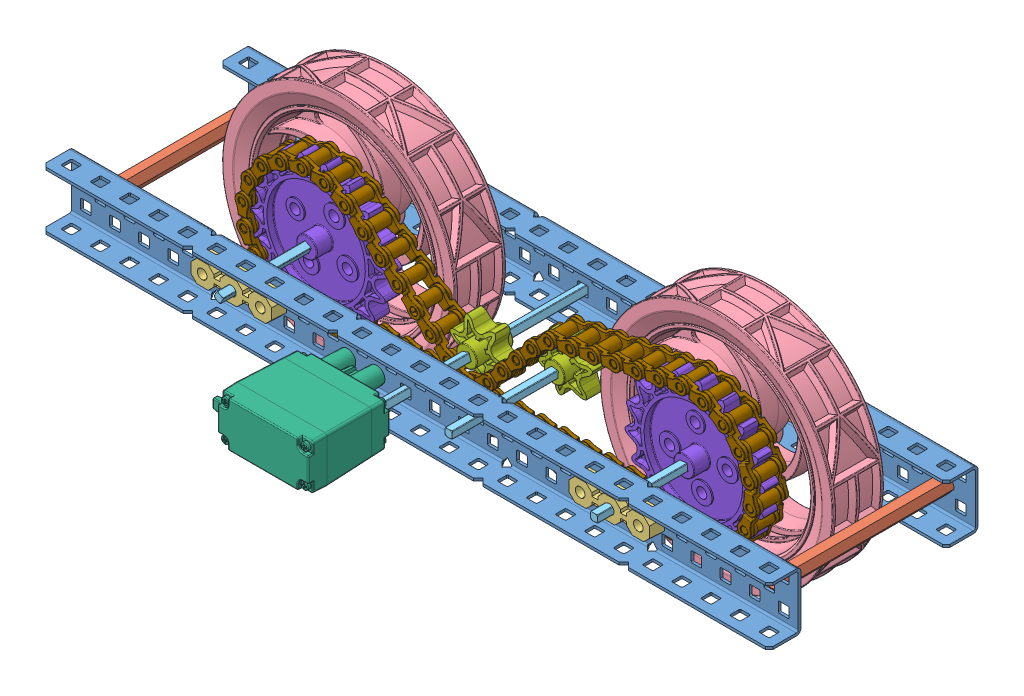
SolidWorks assembly Chassis-NoMates, configuration Default. Lengths in mm.
Overall size (317.5 140.41 141.11).
74 component instances, 9 part files, 0 mates.
Components (placement in the parent):
- BaseUC-4: BaseUC [Default] at (-291.0348 15.6006 0) x (1 0 0) z (0 1 0) size (317.5 13.87 25.4)
- BEAM-3000-7: BEAM-3000 [Default] at (-304.8 12.7 -39.2684) x (1 0 0) z (0 -1 0) size (7.34 77.08 7.34)
- BEAM-3000-8: BEAM-3000 [Default] at (-12.7 12.7 -39.2684) x (-0.63784 -0.770169 0) z (-0.770169 0.63784 0) size (7.34 77.08 7.34)
- BaseUC-7: BaseUC [Default] at (-291.0348 15.6006 -77.3684) x (1 0 0) z (0 1 0) size (317.5 13.87 25.4)
- BEARING-FLAT-5: BEARING-FLAT [Default] at (-49.784 25.4 88.9762) x (0 0 -1) z (0 1 0) size (7.04 35.56 10.16)
- BEARING-FLAT-6: BEARING-FLAT [Default] at (-214.884 25.4 88.9762) x (0 0 -1) z (0 1 0) size (7.04 35.56 10.16)
- BEARING-FLAT-7: BEARING-FLAT [Default] at (-49.784 25.4 11.6078) x (0 0 -1) z (0 1 0) size (7.04 35.56 10.16)
- BEARING-FLAT-8: BEARING-FLAT [Default] at (-214.884 25.4 11.6078) x (0 0 -1) z (0 1 0) size (7.04 35.56 10.16)
- VEX-MEDIUM-WHEEL-3: VEX-MEDIUM-WHEEL [Default] at (-37.1315 -9.2154 -55.044) x (0.998133 0.061083 0) z (0 0 1) size (132.42 132.57 22.31)
- VEX-MEDIUM-WHEEL-4: VEX-MEDIUM-WHEEL [Default] at (-202.5787 -9.8231 -55.044) x (0.998965 0.045481 0) z (0 0 1) size (132.42 132.57 22.31)
- SHAFT-4000-1: SHAFT-4000 [Default] at (-241.3972 12.7906 -38.9947) x (0.456181 0.889887 0) z (0 0 1) size (4.18 4.18 101.81)
- SHAFT-4000-2: SHAFT-4000 [Default] at (-76.5518 12.5236 -38.1812) x (-0.999953 -0.009699 0) z (0 0 1) size (4.18 4.18 101.81)
- SHAFT-4000-3: SHAFT-4000 [Default] at (-132.8293 19.7739 -30.9) size (4.18 4.18 101.81)
- SHAFT-4000-4: SHAFT-4000 [Default] at (-171.4187 6.3323 -30.9) x (-0.963526 -0.267616 0) z (0 0 1) size (4.18 4.18 101.81)
- VEX-2WIRE-MOTOR-1: VEX-2WIRE-MOTOR [Default] at (-182.5798 6.35 43.2) size (46.4 20 51.81)
- sprocket-hs-06-tooth-1: sprocket-hs-06-tooth [Default] at (-171.4187 6.3323 -34.515) x (0.920352 0.391092 0) z (0 0 1) size (21.52 24.74 15.88)
- sprocket-hs-18-tooth-1: sprocket-hs-18-tooth [Default] at (-241.3 12.7 -34.515) x (0.897713 -0.440581 0) z (0 0 1) size (60.62 61.51 15.88)
- sprocket-hs-18-tooth-2: sprocket-hs-18-tooth [Default] at (-76.2 12.7 -34.193) x (0.11417 -0.993461 0) z (0 0 1) size (60.62 61.51 15.88)
- sprocket-hs-06-tooth-2: sprocket-hs-06-tooth [Default] at (-132.8293 19.7739 -34.193) x (0.976296 -0.21644 0) z (0 0 1) size (21.52 24.74 15.88)
- chain-hs-link-1: chain-hs-link [Default] at (-202.2568 17.8785 -29.705) x (0.779269 -0.62669 0) z (0.62669 0.779269 0) size (15.79 14.22 6)
- chain-hs-link-3: chain-hs-link [Default] at (-209.8931 24.0197 -29.705) x (0.779269 -0.62669 0) z (0.62669 0.779269 0) size (15.79 14.22 6)
- chain-hs-link-4: chain-hs-link [Default] at (-217.5294 30.1608 -29.705) x (0.779269 -0.62669 0) z (0.62669 0.779269 0) size (15.79 14.22 6)
- chain-hs-link-5: chain-hs-link [Default] at (-225.2134 36.2422 -29.705) x (0.784132 -0.620594 0) z (0.620594 0.784132 0) size (15.79 14.22 6)
- chain-hs-link-6: chain-hs-link [Default] at (-234.1156 40.3382 -29.705) x (0.908451 -0.417991 0) z (0.417991 0.908451 0) size (15.79 14.22 6)
- chain-hs-link-7: chain-hs-link [Default] at (-243.879 41.1761 -29.705) x (0.996338 -0.0855 0) z (0.0855 0.996338 0) size (15.79 14.22 6)
- chain-hs-link-8: chain-hs-link [Default] at (-253.3489 38.6566 -29.705) x (0.966384 0.257104 0) z (-0.257104 0.966384 0) size (15.79 14.22 6)
- chain-hs-link-9: chain-hs-link [Default] at (-261.4052 33.0779 -29.705) x (0.822131 0.569299 0) z (-0.569299 0.822131 0) size (15.79 14.22 6)
- chain-hs-link-10: chain-hs-link [Default] at (-267.0951 25.0997 -29.705) x (0.58064 0.81416 0) z (-0.81416 0.58064 0) size (15.79 14.22 6)
- chain-hs-link-11: chain-hs-link [Default] at (-269.7456 15.6656 -29.705) x (0.270475 0.962727 0) z (-0.962727 0.270475 0) size (15.79 14.22 6)
- chain-hs-link-12: chain-hs-link [Default] at (-269.0432 5.8915 -29.705) x (-0.071681 0.997428 0) z (-0.997428 -0.071681 0) size (15.79 14.22 6)
- chain-hs-link-13: chain-hs-link [Default] at (-265.0709 -3.0666 -29.705) x (-0.405359 0.914158 0) z (-0.914158 -0.405359 0) size (15.79 14.22 6)
- chain-hs-link-14: chain-hs-link [Default] at (-258.2987 -10.1493 -29.705) x (-0.691093 0.722766 0) z (-0.722766 -0.691093 0) size (15.79 14.22 6)
- chain-hs-link-15: chain-hs-link [Default] at (-249.5274 -14.5187 -29.705) x (-0.895088 0.44589 0) z (-0.44589 -0.895088 0) size (15.79 14.22 6)
- chain-hs-link-16: chain-hs-link [Default] at (-239.8 -15.7032 -29.705) x (-0.992667 0.120879 0) z (-0.120879 -0.992667 0) size (15.79 14.22 6)
- chain-hs-link-17: chain-hs-link [Default] at (-230.0006 -15.7032 -29.705) x (-1 0 0) z (0 -1 0) size (15.79 14.22 6)
- chain-hs-link-18: chain-hs-link [Default] at (-220.2013 -15.7032 -29.705) x (-1 0 0) z (0 -1 0) size (15.79 14.22 6)
- chain-hs-link-19: chain-hs-link [Default] at (-210.402 -15.7032 -29.705) x (-1 0 0) z (0 -1 0) size (15.79 14.22 6)
- chain-hs-link-20: chain-hs-link [Default] at (-200.6027 -15.7032 -29.705) x (-1 0 0) z (0 -1 0) size (15.79 14.22 6)
- chain-hs-link-21: chain-hs-link [Default] at (-190.8033 -15.7032 -29.705) x (-1 0 0) z (0 -1 0) size (15.79 14.22 6)
- chain-hs-link-22: chain-hs-link [Default] at (-181.004 -15.7032 -29.705) x (-1 0 0) z (0 -1 0) size (15.79 14.22 6)
- chain-hs-link-23: chain-hs-link [Default] at (-171.2047 -15.7032 -29.705) x (-1 0 0) z (0 -1 0) size (15.79 14.22 6)
- chain-hs-link-24: chain-hs-link [Default] at (-161.4054 -15.7032 -29.705) x (-1 0 0) z (0 -1 0) size (15.79 14.22 6)
- chain-hs-link-25: chain-hs-link [Default] at (-151.6061 -15.7032 -29.705) x (-1 0 0) z (0 -1 0) size (15.79 14.22 6)
- chain-hs-link-26: chain-hs-link [Default] at (-141.8067 -15.7032 -29.705) x (-1 0 0) z (0 -1 0) size (15.79 14.22 6)
- chain-hs-link-27: chain-hs-link [Default] at (-132.0074 -15.7032 -29.705) x (-1 0 0) z (0 -1 0) size (15.79 14.22 6)
- chain-hs-link-28: chain-hs-link [Default] at (-122.2081 -15.7032 -29.705) x (-1 0 0) z (0 -1 0) size (15.79 14.22 6)
- chain-hs-link-29: chain-hs-link [Default] at (-112.4088 -15.7032 -29.705) x (-1 0 0) z (0 -1 0) size (15.79 14.22 6)
- chain-hs-link-30: chain-hs-link [Default] at (-102.6094 -15.7032 -29.705) x (-1 0 0) z (0 -1 0) size (15.79 14.22 6)
- chain-hs-link-31: chain-hs-link [Default] at (-92.8101 -15.7032 -29.705) x (-1 0 0) z (0 -1 0) size (15.79 14.22 6)
- chain-hs-link-32: chain-hs-link [Default] at (-83.0108 -15.7032 -29.705) x (-1 0 0) z (0 -1 0) size (15.79 14.22 6)
- chain-hs-link-33: chain-hs-link [Default] at (-73.2127 -15.5457 -29.705) x (-0.999871 -0.016075 0) z (0.016075 -0.999871 0) size (15.79 14.22 6)
- chain-hs-link-34: chain-hs-link [Default] at (-63.7916 -12.8494 -29.705) x (-0.961403 -0.275144 0) z (0.275144 -0.961403 0) size (15.79 14.22 6)
- chain-hs-link-35: chain-hs-link [Default] at (-55.8475 -7.1121 -29.705) x (-0.810681 -0.585488 0) z (0.585488 -0.810681 0) size (15.79 14.22 6)
- chain-hs-link-36: chain-hs-link [Default] at (-50.326 0.9836 -29.705) x (-0.563464 -0.826141 0) z (0.826141 -0.563464 0) size (15.79 14.22 6)
- chain-hs-link-37: chain-hs-link [Default] at (-47.8842 10.4738 -29.705) x (-0.249177 -0.968458 0) z (0.968458 -0.249177 0) size (15.79 14.22 6)
- chain-hs-link-38: chain-hs-link [Default] at (-48.8129 20.229 -29.705) x (0.09477 -0.995499 0) z (0.995499 0.09477 0) size (15.79 14.22 6)
- chain-hs-link-39: chain-hs-link [Default] at (-53.0014 29.0881 -29.705) x (0.427436 -0.904046 0) z (0.904046 0.427436 0) size (15.79 14.22 6)
- chain-hs-link-40: chain-hs-link [Default] at (-59.9513 35.9964 -29.705) x (0.709224 -0.704984 0) z (0.704984 0.709224 0) size (15.79 14.22 6)
- chain-hs-link-41: chain-hs-link [Default] at (-68.8353 40.1318 -29.705) x (0.906593 -0.422007 0) z (0.422007 0.906593 0) size (15.79 14.22 6)
- chain-hs-link-42: chain-hs-link [Default] at (-78.596 41.002 -29.705) x (0.99605 -0.088798 0) z (0.088798 0.99605 0) size (15.79 14.22 6)
- chain-hs-link-43: chain-hs-link [Default] at (-88.2359 39.2421 -29.705) x (0.983741 0.179593 0) z (-0.179593 0.983741 0) size (15.79 14.22 6)
- chain-hs-link-44: chain-hs-link [Default] at (-97.8402 37.2967 -29.705) x (0.980096 0.198523 0) z (-0.198523 0.980096 0) size (15.79 14.22 6)
- chain-hs-link-45: chain-hs-link [Default] at (-107.4445 35.3513 -29.705) x (0.980096 0.198523 0) z (-0.198523 0.980096 0) size (15.79 14.22 6)
- chain-hs-link-46: chain-hs-link [Default] at (-117.0488 33.4059 -29.705) x (0.980096 0.198523 0) z (-0.198523 0.980096 0) size (15.79 14.22 6)
- chain-hs-link-47: chain-hs-link [Default] at (-126.6531 31.4605 -29.705) x (0.980096 0.198523 0) z (-0.198523 0.980096 0) size (15.79 14.22 6)
- chain-hs-link-48: chain-hs-link [Default] at (-136.237 29.4174 -29.705) x (0.978023 0.208496 0) z (-0.208496 0.978023 0) size (15.79 14.22 6)
- chain-hs-link-49: chain-hs-link [Default] at (-143.5879 22.9374 -29.705) x (0.750143 0.661276 0) z (-0.661276 0.750143 0) size (15.79 14.22 6)
- chain-hs-link-50: chain-hs-link [Default] at (-149.9643 15.4963 -29.705) x (0.650693 0.759341 0) z (-0.759341 0.650693 0) size (15.79 14.22 6)
- chain-hs-link-51: chain-hs-link [Default] at (-156.3406 8.0553 -29.705) x (0.650693 0.759341 0) z (-0.759341 0.650693 0) size (15.79 14.22 6)
- chain-hs-link-52: chain-hs-link [Default] at (-162.717 0.6143 -29.705) x (0.650693 0.759341 0) z (-0.759341 0.650693 0) size (15.79 14.22 6)
- chain-hs-link-53: chain-hs-link [Default] at (-171.3641 -3.9958 -29.705) x (0.882425 0.470452 0) z (-0.470452 0.882425 0) size (15.79 14.22 6)
- chain-hs-link-54: chain-hs-link [Default] at (-180.2347 0.1683 -29.705) x (0.905222 -0.42494 0) z (0.42494 0.905222 0) size (15.79 14.22 6)
- chain-hs-link-55: chain-hs-link [Default] at (-187.871 6.3094 -29.705) x (0.779269 -0.62669 0) z (0.62669 0.779269 0) size (15.79 14.22 6)
- chain-hs-link-56: chain-hs-link [Default] at (-195.5073 12.4505 -29.705) x (0.779269 -0.62669 0) z (0.62669 0.779269 0) size (15.79 14.22 6)
